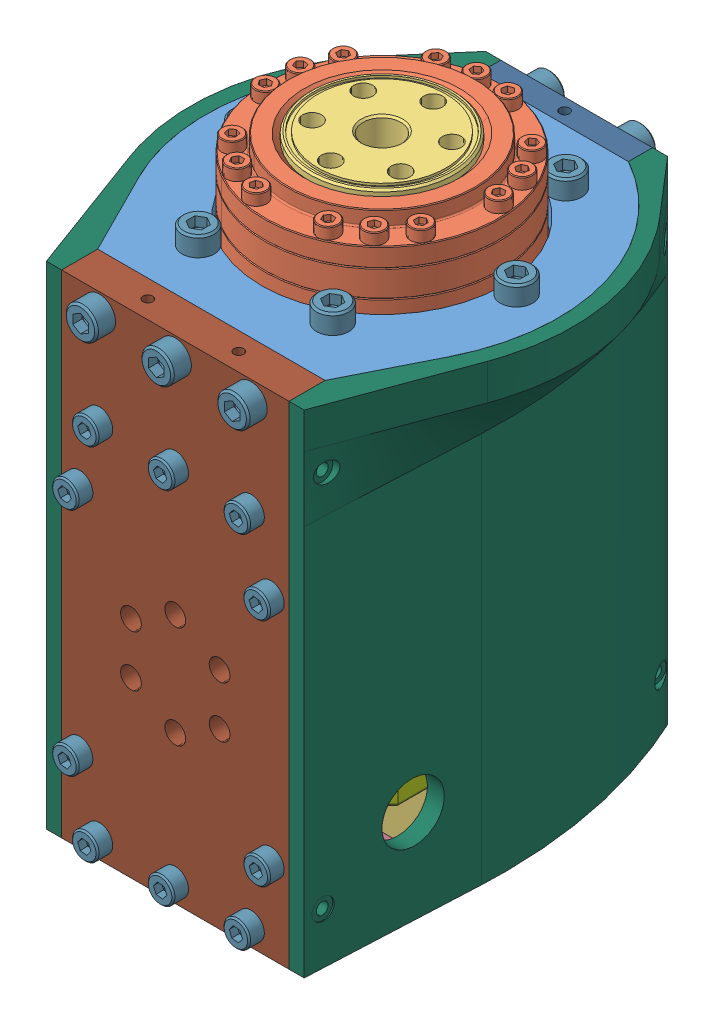
SolidWorks assembly DEC_asm, configuration Default. Lengths in mm.
Overall size (107.92 151.34 115.88).
57 component instances, 15 part files, 101 mates.
Components (placement in the parent):
- DEC_gearbox_mount-1: DEC_gearbox_mount [Default] at (31.2065 45.5966 71.2738) size (92.96 9.53 90)
- CSF-17-XXX-2UH.stp-1: CSF-17-XXX-2UH.stp [Default] at (31.2065 69.8341 71.2738) x (0 -1 0) z (0.5 0 -0.866025) size (45 79 79)
  - CSF-17-2UH HOUSING.stp-1: CSF-17-2UH HOUSING.stp [Default] at origin size (38.5 79 79)
  - CSF-17-2UH OUTPUT.stp-1: CSF-17-2UH OUTPUT.stp [Default] at (0 -0.0003 0) x (1 0.000008 0) z (0 0 1) size (39 44 44)
  - CSF-17-2A-R OLDHAM COUPLING.stp-1: CSF-17-2A-R OLDHAM COUPLING.stp [Default] at (45 0 0) x (1 0 0) z (0 0 -1) size (19.5 37 37)
  - 1715063_1715063.stp-1: 1715063_1715063.stp [Default] at (42 0 9) x (0 0 -1) z (-0.999997 -0.002366 0) size (4 3 3)
  - 1715063_1715063.stp-2: 1715063_1715063.stp [Default] at (42 -9 0) x (0 1 0) z (0.378269 0 0.925696) size (4 3 3)
  - 17 WG BEARING.stp-1: 17 WG BEARING.stp [Default] at (32.285 0 0) size (6.67 42 42)
- Nema17_27_1-1: Nema17_27_1 [Default] at (-8.1003 -74.3741 116.9592) x (1 0 0) z (0 1 0) size (42.4 43.16 103.01)
  - 6627T91_Stepper Motor-1: 6627T91_Stepper Motor [6627T91] at (39.3069 45.6854 45.8837) size (42.4 43.16 74.04)
  - Planatary_Gearbox_27_1-1: Planatary_Gearbox_27_1 [Default] at (39.3069 45.6854 56.8707) size (42.1 42.1 55)
- DEC_planetary_mount-1: DEC_planetary_mount [Default] at (31.2065 20.5966 71.2738) x (1 0 0) z (0 1 0) size (60 90 6.2)
- DEC_top_plate-1: DEC_top_plate [Default] at (31.2065 -29.6409 23.0988) x (-1 0 0) z (0 -1 0) size (40 6.35 129.76)
- DEC_bottom_plate-1: DEC_bottom_plate [Default] at (31.2065 -29.6409 121.0388) x (-1 0 0) z (0 -1 0) size (60 9.53 129.76)
- DEC_middle_support_v2-1: DEC_middle_support_v2 [Default] at (31.2065 -74.4034 71.2738) x (-1 0 0) z (0 -1 0) size (60 90 6.2)
- support_triangle-1: support_triangle [Default] at (51.6815 -71.3034 116.2738) x (0 0 -1) z (1 0 0) size (18 18 9.53)
- support_triangle-2: support_triangle [Default] at (41.6815 -71.3034 26.2738) x (0 1 0) z (1 0 0) size (18 18 9.53)
- support_triangle-3: support_triangle [Default] at (1.2065 -71.3034 116.2738) x (0 0 -1) z (1 0 0) size (18 18 9.53)
- support_triangle-4: support_triangle [Default] at (11.2065 -71.3034 26.2738) x (0 1 0) z (1 0 0) size (18 18 9.53)
- support_triangle-5: support_triangle [Default] at (41.6815 17.4966 26.2738) x (0 0 1) z (1 0 0) size (18 18 9.53)
- support_triangle-6: support_triangle [Default] at (1.2065 17.4966 116.2738) x (0 -1 0) z (1 0 0) size (18 18 9.53)
- support_triangle-7: support_triangle [Default] at (51.6815 17.4966 116.2738) x (0 -1 0) z (1 0 0) size (18 18 9.53)
- support_triangle-8: support_triangle [Default] at (11.2065 17.4966 26.2738) x (0 0 1) z (1 0 0) size (18 18 9.53)
- socket head cap screw_am-4: socket head cap screw_am [B18.3.1M - 4 x 0.7 x 12 Hex SHCS -- 12NHX] at (43.2065 -74.4034 15.9238) x (0 0 1) z (-1 0 0) size (16 7 7)
- socket head cap screw_am-5: socket head cap screw_am [B18.3.1M - 4 x 0.7 x 12 Hex SHCS -- 12NHX] at (19.2065 20.5966 15.9238) x (0 0 1) z (-0.77104 0.636787 0) size (16 7 7)
- socket head cap screw_am-6: socket head cap screw_am [B18.3.1M - 4 x 0.7 x 12 Hex SHCS -- 12NHX] at (46.444 -57.3034 15.9238) x (0 0 1) z (-1 0 0) size (16 7 7)
- socket head cap screw_am-7: socket head cap screw_am [B18.3.1M - 4 x 0.7 x 12 Hex SHCS -- 12NHX] at (19.2065 -74.4034 15.9238) x (0 0 1) z (-1 0 0) size (16 7 7)
- socket head cap screw_am-8: socket head cap screw_am [B18.3.1M - 4 x 0.7 x 12 Hex SHCS -- 12NHX] at (15.969 3.4966 15.9238) x (0 0 1) z (-1 0 0) size (16 7 7)
- socket head cap screw_am-9: socket head cap screw_am [B18.3.1M - 4 x 0.7 x 12 Hex SHCS -- 12NHX] at (15.969 -57.3034 15.9238) x (0 0 1) z (-1 0 0) size (16 7 7)
- socket head cap screw_am-10: socket head cap screw_am [B18.3.1M - 4 x 0.7 x 12 Hex SHCS -- 12NHX] at (43.2065 20.5966 15.9238) x (0 0 1) z (-1 0 0) size (16 7 7)
- socket head cap screw_am-11: socket head cap screw_am [B18.3.1M - 4 x 0.7 x 12 Hex SHCS -- 12NHX] at (46.444 3.4966 15.9238) x (0 0 1) z (-1 0 0) size (16 7 7)
- socket head cap screw_am-12: socket head cap screw_am [B18.3.1M - 5 x 0.8 x 12 Hex SHCS -- 12NHX] at (43.2065 45.5966 14.9238) x (0 0 1) z (-1 0 0) size (17 8.5 8.5)
- socket head cap screw_am-13: socket head cap screw_am [B18.3.1M - 5 x 0.8 x 12 Hex SHCS -- 12NHX] at (19.2065 45.5966 14.9238) x (0 0 1) z (-1 0 0) size (17 8.5 8.5)
- socket head cap screw_am-14: socket head cap screw_am [B18.3.1M - 5 x 0.8 x 12 Hex SHCS -- 12NHX] at (51.2065 45.5966 130.8038) x (0 0 -1) z (1 0 0) size (17 8.5 8.5)
- socket head cap screw_am-15: socket head cap screw_am [B18.3.1M - 5 x 0.8 x 12 Hex SHCS -- 12NHX] at (11.2065 45.5966 130.8038) x (0 0 -1) z (1 0 0) size (17 8.5 8.5)
- socket head cap screw_am-16: socket head cap screw_am [B18.3.1M - 5 x 0.8 x 12 Hex SHCS -- 12NHX] at (31.2065 45.5966 130.8038) x (0 0 -1) z (1 0 0) size (17 8.5 8.5)
- socket head cap screw_am-17: socket head cap screw_am [B18.3.1M - 4 x 0.7 x 12 Hex SHCS -- 12NHX] at (31.2065 20.5966 129.8038) x (0 0 -1) z (0.923728 0.383049 0) size (16 7 7)
- socket head cap screw_am-18: socket head cap screw_am [B18.3.1M - 4 x 0.7 x 12 Hex SHCS -- 12NHX] at (51.2065 20.5966 129.8038) x (0 0 -1) z (0.923728 0.383049 0) size (16 7 7)
- socket head cap screw_am-19: socket head cap screw_am [B18.3.1M - 4 x 0.7 x 12 Hex SHCS -- 12NHX] at (5.969 3.4966 129.8038) x (0 0 -1) z (0.923728 0.383049 0) size (16 7 7)
- socket head cap screw_am-20: socket head cap screw_am [B18.3.1M - 4 x 0.7 x 12 Hex SHCS -- 12NHX] at (56.444 3.4966 129.8038) x (0 0 -1) z (0.923728 0.383049 0) size (16 7 7)
- socket head cap screw_am-21: socket head cap screw_am [B18.3.1M - 4 x 0.7 x 12 Hex SHCS -- 12NHX] at (5.969 -57.3034 129.8038) x (0 0 -1) z (0.923728 0.383049 0) size (16 7 7)
- socket head cap screw_am-22: socket head cap screw_am [B18.3.1M - 4 x 0.7 x 12 Hex SHCS -- 12NHX] at (56.444 -57.3034 129.8038) x (0 0 -1) z (0.923728 0.383049 0) size (16 7 7)
- socket head cap screw_am-23: socket head cap screw_am [B18.3.1M - 4 x 0.7 x 12 Hex SHCS -- 12NHX] at (11.2065 -74.4034 129.8038) x (0 0 -1) z (0.923728 0.383049 0) size (16 7 7)
- socket head cap screw_am-24: socket head cap screw_am [B18.3.1M - 4 x 0.7 x 12 Hex SHCS -- 12NHX] at (51.2065 -74.4034 129.8038) x (0 0 -1) z (0.923728 0.383049 0) size (16 7 7)
- socket head cap screw_am-25: socket head cap screw_am [B18.3.1M - 4 x 0.7 x 12 Hex SHCS -- 12NHX] at (11.2065 20.5966 129.8038) x (0 0 -1) z (0.923728 0.383049 0) size (16 7 7)
- socket head cap screw_am-26: socket head cap screw_am [B18.3.1M - 4 x 0.7 x 12 Hex SHCS -- 12NHX] at (31.2065 -74.4034 129.8038) x (0 0 -1) z (0.923728 0.383049 0) size (16 7 7)
- socket head cap screw_am-27: socket head cap screw_am [B18.3.1M - 4 x 0.7 x 12 Hex SHCS -- 12NHX] at (46.444 -81.5034 40.2738) x (0 1 0) z (-0.56381 0 -0.825904) size (16 7 7)
- socket head cap screw_am-28: socket head cap screw_am [B18.3.1M - 4 x 0.7 x 12 Hex SHCS -- 12NHX] at (15.969 -81.5034 40.2738) x (0 1 0) z (-0.56381 0 -0.825904) size (16 7 7)
- socket head cap screw_am-29: socket head cap screw_am [B18.3.1M - 4 x 0.7 x 12 Hex SHCS -- 12NHX] at (5.969 -81.5034 102.2738) x (0 1 0) z (-0.56381 0 -0.825904) size (16 7 7)
- socket head cap screw_am-30: socket head cap screw_am [B18.3.1M - 4 x 0.7 x 12 Hex SHCS -- 12NHX] at (56.444 -81.5034 102.2738) x (0 1 0) z (-0.56381 0 -0.825904) size (16 7 7)
- socket head cap screw_am-31: socket head cap screw_am [B18.3.1M - 5 x 0.8 x 12 Hex SHCS -- 12NHX] at (48.9565 55.3591 102.0177) x (0 -1 0) z (1 0 0) size (17 8.5 8.5)
- socket head cap screw_am-32: socket head cap screw_am [B18.3.1M - 5 x 0.8 x 12 Hex SHCS -- 12NHX] at (13.4565 55.3591 102.0177) x (0 -1 0) z (1 0 0) size (17 8.5 8.5)
- socket head cap screw_am-33: socket head cap screw_am [B18.3.1M - 5 x 0.8 x 12 Hex SHCS -- 12NHX] at (48.9565 55.3591 40.5299) x (0 -1 0) z (1 0 0) size (17 8.5 8.5)
- socket head cap screw_am-34: socket head cap screw_am [B18.3.1M - 5 x 0.8 x 12 Hex SHCS -- 12NHX] at (-4.2935 55.3591 71.2738) x (0 -1 0) z (1 0 0) size (17 8.5 8.5)
- socket head cap screw_am-35: socket head cap screw_am [B18.3.1M - 5 x 0.8 x 12 Hex SHCS -- 12NHX] at (13.4565 55.3591 40.5299) x (0 -1 0) z (1 0 0) size (17 8.5 8.5)
- socket head cap screw_am-36: socket head cap screw_am [B18.3.1M - 5 x 0.8 x 12 Hex SHCS -- 12NHX] at (66.7065 55.3591 71.2738) x (0 -1 0) z (1 0 0) size (17 8.5 8.5)
- Part1^DEC_asm-1: Part1^DEC_asm [Default] at origin size (101.02 129.76 105.9) (virtual)
Mates (geometry in assembly coordinates):
- Coincident3: coincident anti-aligned: plane of RA_gearbox_mount-1 through (11.2065 50.3591 26.2738) normal (0 0 -1); plane of DEC_top_plate-1 through (31.2065 -29.6409 26.2738) normal (0 0 1)
- Concentric8: concentric aligned: cylinder of RA_gearbox_mount-1 through (31.2065 45.5966 108.2738) axis (0 0 1) radius 2.15; cylinder of DEC_bottom_plate-1 through (31.2065 45.5966 114.6888) axis (0 0 1) radius 2.75
- Concentric9: concentric aligned: cylinder of RA_planetary_mount-1 through (31.2065 20.5966 108.2738) axis (0 0 1) radius 1.7; cylinder of DEC_bottom_plate-1 through (31.2065 20.5966 114.6888) axis (0 0 1) radius 2.2
- Coincident4: coincident anti-aligned: plane of RA_planetary_mount-1 through (1.2065 23.6966 116.2738) normal (0 0 1); plane of DEC_bottom_plate-1 through (31.2065 -29.6409 116.2738) normal (0 0 -1)
- Concentric10: concentric aligned: cylinder of DEC_bottom_plate-1 through (11.2065 -74.4034 114.6888) axis (0 0 1) radius 2.2; cylinder of DEC_middle_support_v2-1 through (11.2065 -74.4034 108.2738) axis (0 0 1) radius 1.7
- Concentric11: concentric aligned: cylinder of DEC_bottom_plate-1 through (51.2065 -74.4034 114.6888) axis (0 0 1) radius 2.2; cylinder of DEC_middle_support_v2-1 through (51.2065 -74.4034 108.2738) axis (0 0 1) radius 1.7
- Coincident5: coincident anti-aligned: plane of DEC_bottom_plate-1 through (31.2065 -29.6409 116.2738) normal (0 0 -1); plane of DEC_middle_support_v2-1 through (61.2065 -77.5034 116.2738) normal (0 0 1)
- Concentric14: concentric anti-aligned: cylinder of RA_gearbox_mount-1 through (43.2065 45.5966 34.2738) axis (0 0 -1) radius 2.15; cylinder of DEC_top_plate-1 through (43.2065 45.5966 16.7488) axis (0 0 1) radius 2.75
- Concentric15: concentric anti-aligned: cylinder of RA_planetary_mount-1 through (19.2065 20.5966 34.2738) axis (0 0 -1) radius 1.7; cylinder of DEC_top_plate-1 through (19.2065 20.5966 16.7488) axis (0 0 1) radius 2.2
- Coincident6: coincident anti-aligned: plane of RA_gearbox_mount-1 through (26.2065 40.8341 71.2738) normal (0 -1 0); plane of CSF-17-XXX-2UH.stp-1/CSF-17-2UH HOUSING.stp-1 through (3.5803 40.8341 55.3238) normal (0 1 0)
- Concentric16: concentric anti-aligned: cylinder of RA_gearbox_mount-1 through (13.4565 34.6116 40.5299) axis (0 1 0) radius 2.2; cylinder of CSF-17-XXX-2UH.stp-1/CSF-17-2UH HOUSING.stp-1 through (13.4565 32.8341 40.5299) axis (0 -1 0) radius 1.65
- Concentric18: concentric anti-aligned: cylinder of RA_gearbox_mount-1 through (-4.2935 34.6116 71.2738) axis (0 1 0) radius 2.2; cylinder of CSF-17-XXX-2UH.stp-1/CSF-17-2UH HOUSING.stp-1 through (-4.2935 32.8341 71.2738) axis (0 -1 0) radius 1.65
- Concentric19: concentric anti-aligned: cylinder of RA_gearbox_mount-1 through (19.2065 45.5966 34.2738) axis (0 0 -1) radius 2.15; cylinder of DEC_top_plate-1 through (19.2065 45.5966 16.7488) axis (0 0 1) radius 2.75
- Coincident7: coincident anti-aligned: plane of RA_planetary_mount-1 through (11.2065 23.6966 26.2738) normal (0 0 -1); plane of DEC_top_plate-1 through (31.2065 -29.6409 26.2738) normal (0 0 1)
- Concentric20: concentric anti-aligned: cylinder of DEC_top_plate-1 through (19.2065 -74.4034 16.7488) axis (0 0 1) radius 2.2; cylinder of DEC_middle_support_v2-1 through (19.2065 -74.4034 34.2738) axis (0 0 -1) radius 1.7
- Concentric21: concentric anti-aligned: cylinder of DEC_top_plate-1 through (43.2065 -74.4034 16.7488) axis (0 0 1) radius 2.2; cylinder of DEC_middle_support_v2-1 through (43.2065 -74.4034 34.2738) axis (0 0 -1) radius 1.7
- Concentric22: concentric aligned: cylinder of Nema17_27_1-1/Planatary_Gearbox_27_1-1 through (21.307 7.4966 61.3743) axis (0 1 0) radius 1.5; cylinder of RA_planetary_mount-1 through (21.307 13.8196 61.3743) axis (0 1 0) radius 1.3
- Concentric283: concentric aligned: circle of Nema17_27_1-1/Planatary_Gearbox_27_1-1; cylinder of DEC_planetary_mount-1 through (21.307 13.8196 81.1733) axis (0 1 0) radius 1.3
- Coincident9: coincident anti-aligned: plane of Nema17_27_1-1/Planatary_Gearbox_27_1-1 through (31.2065 17.4966 71.2738) normal (0 1 0); plane of RA_planetary_mount-1 through (31.2065 17.4966 71.2738) normal (0 -1 0)
- Concentric23: concentric anti-aligned: cylinder of DEC_bottom_plate-1 through (56.444 -57.3034 132.0264) axis (0 0 -1) radius 2.2; cylinder of support_triangle-1 through (56.444 -57.3034 102.617) axis (0 0 1) radius 2
- Concentric24: concentric aligned: cylinder of DEC_middle_support_v2-1 through (56.444 -65.0809 102.2738) axis (0 -1 0) radius 2.2; cylinder of support_triangle-1 through (56.444 -57.6465 102.2738) axis (0 -1 0) radius 2
- Concentric25: concentric anti-aligned: circle of RA_middle_support-1; cylinder of support_triangle-2 through (46.444 -57.6465 40.2738) axis (0 -1 0) radius 2
- Concentric26: concentric aligned: cylinder of DEC_top_plate-1 through (46.444 -57.3034 32.4964) axis (0 0 -1) radius 2.2; cylinder of support_triangle-2 through (46.444 -57.3034 39.9307) axis (0 0 -1) radius 2
- Concentric27: concentric anti-aligned: cylinder of DEC_bottom_plate-1 through (5.969 -57.3034 132.0264) axis (0 0 -1) radius 2.2; cylinder of support_triangle-3 through (5.969 -57.3034 102.617) axis (0 0 1) radius 2
- Concentric28: concentric aligned: cylinder of DEC_middle_support_v2-1 through (5.969 -65.0809 102.2738) axis (0 -1 0) radius 2.2; cylinder of support_triangle-3 through (5.969 -57.6465 102.2738) axis (0 -1 0) radius 2
- Concentric29: concentric aligned: cylinder of DEC_top_plate-1 through (15.969 -57.3034 32.4964) axis (0 0 -1) radius 2.2; cylinder of support_triangle-4 through (15.969 -57.3034 39.9307) axis (0 0 -1) radius 2
- Concentric30: concentric aligned: cylinder of DEC_middle_support_v2-1 through (15.969 -65.0809 40.2738) axis (0 -1 0) radius 2.2; cylinder of support_triangle-4 through (15.969 -57.6465 40.2738) axis (0 -1 0) radius 2
- Concentric31: concentric anti-aligned: cylinder of RA_planetary_mount-1 through (5.969 11.2741 102.2738) axis (0 1 0) radius 2.2; circle of support_triangle-6
- Concentric32: concentric anti-aligned: cylinder of DEC_bottom_plate-1 through (5.969 3.4966 132.0264) axis (0 0 -1) radius 2.2; circle of support_triangle-6
- Concentric33: concentric anti-aligned: cylinder of DEC_bottom_plate-1 through (56.444 3.4966 132.0264) axis (0 0 -1) radius 2.2; circle of support_triangle-7
- Concentric34: concentric aligned: cylinder of RA_planetary_mount-1 through (56.444 11.2741 102.2738) axis (0 1 0) radius 2.2; cylinder of support_triangle-7 through (56.444 3.8397 102.2738) axis (0 1 0) radius 2
- Concentric36: concentric aligned: cylinder of RA_planetary_mount-1 through (46.444 11.2741 40.2738) axis (0 1 0) radius 2.2; cylinder of support_triangle-5 through (46.444 3.8397 40.2738) axis (0 1 0) radius 2
- Concentric37: concentric aligned: cylinder of DEC_top_plate-1 through (46.444 3.4966 32.4964) axis (0 0 -1) radius 2.2; circle of support_triangle-5
- Concentric38: concentric aligned: cylinder of DEC_top_plate-1 through (15.969 3.4966 32.4964) axis (0 0 -1) radius 2.2; cylinder of support_triangle-8 through (15.969 3.4966 39.9307) axis (0 0 -1) radius 2
- Concentric39: concentric anti-aligned: cylinder of RA_planetary_mount-1 through (15.969 11.2741 40.2738) axis (0 1 0) radius 2.2; circle of support_triangle-8
- Concentric250: concentric anti-aligned: cylinder of DEC_top_plate-1 through (19.2065 20.5966 16.7488) axis (0 0 1) radius 2.2; cylinder of socket head cap screw_am-5 through (19.2065 20.5966 -15.8262) axis (0 0 -1) radius 2
- Coincident219: coincident aligned: plane of DEC_top_plate-1 through (31.2065 -29.6409 19.9238) normal (0 0 -1); circle of socket head cap screw_am-5
- Coincident220: coincident aligned: plane of socket head cap screw_am-4 through (43.2065 -72.7934 31.9238) normal (0 0 1); plane of socket head cap screw_am-7 through (19.2065 -72.7934 31.9238) normal (0 0 1)
- Coincident221: coincident aligned: plane of socket head cap screw_am-6 through (46.444 -55.6934 31.9238) normal (0 0 1); plane of socket head cap screw_am-7 through (19.2065 -72.7934 31.9238) normal (0 0 1)
- Coincident222: coincident aligned: plane of socket head cap screw_am-6 through (46.444 -55.6934 31.9238) normal (0 0 1); plane of socket head cap screw_am-9 through (15.969 -55.6934 31.9238) normal (0 0 1)
- Coincident223: coincident aligned: plane of socket head cap screw_am-9 through (15.969 -55.6934 31.9238) normal (0 0 1); plane of socket head cap screw_am-11 through (46.444 5.1066 31.9238) normal (0 0 1)
- Coincident224: coincident aligned: plane of socket head cap screw_am-8 through (15.969 5.1066 31.9238) normal (0 0 1); plane of socket head cap screw_am-11 through (46.444 5.1066 31.9238) normal (0 0 1)
- Coincident225: coincident aligned: plane of socket head cap screw_am-8 through (15.969 5.1066 31.9238) normal (0 0 1); plane of socket head cap screw_am-10 through (43.2065 22.2066 31.9238) normal (0 0 1)
- Coincident226: coincident anti-aligned: plane of DEC_top_plate-1 through (31.2065 -29.6409 19.9238) normal (0 0 -1); plane of socket head cap screw_am-10 through (43.2065 24.0966 19.9238) normal (0 0 1)
- Concentric251: concentric anti-aligned: circle of DEC_top_plate-1; cylinder of socket head cap screw_am-10 through (43.2065 20.5966 -15.8262) axis (0 0 -1) radius 3.5
- Concentric252: concentric aligned: circle of DEC_top_plate-1; cylinder of socket head cap screw_am-8 through (15.969 3.4966 -15.8262) axis (0 0 -1) radius 2
- Concentric253: concentric aligned: cylinder of DEC_top_plate-1 through (46.444 3.4966 32.4964) axis (0 0 -1) radius 2.2; cylinder of socket head cap screw_am-11 through (46.444 3.4966 -15.8262) axis (0 0 -1) radius 2
- Concentric254: concentric aligned: circle of DEC_top_plate-1; cylinder of socket head cap screw_am-9 through (15.969 -57.3034 -15.8262) axis (0 0 -1) radius 2
- Concentric255: concentric aligned: cylinder of DEC_top_plate-1 through (46.444 -57.3034 32.4964) axis (0 0 -1) radius 2.2; cylinder of socket head cap screw_am-6 through (46.444 -57.3034 -15.8262) axis (0 0 -1) radius 2
- Concentric256: concentric anti-aligned: circle of DEC_top_plate-1; cylinder of socket head cap screw_am-7 through (19.2065 -74.4034 -15.8262) axis (0 0 -1) radius 2
- Concentric257: concentric anti-aligned: circle of DEC_top_plate-1; cylinder of socket head cap screw_am-4 through (43.2065 -74.4034 -15.8262) axis (0 0 -1) radius 2
- Coincident227: coincident aligned: plane of socket head cap screw_am-12 through (43.2065 47.6516 31.9238) normal (0 0 1); plane of socket head cap screw_am-13 through (19.2065 47.6516 31.9238) normal (0 0 1)
- Coincident228: coincident anti-aligned: plane of DEC_top_plate-1 through (31.2065 -29.6409 19.9238) normal (0 0 -1); plane of socket head cap screw_am-13 through (19.2065 49.8466 19.9238) normal (0 0 1)
- Concentric258: concentric anti-aligned: cylinder of DEC_top_plate-1 through (19.2065 45.5966 16.7488) axis (0 0 1) radius 2.75; cylinder of socket head cap screw_am-13 through (19.2065 45.5966 -16.8262) axis (0 0 -1) radius 4.25
- Concentric259: concentric anti-aligned: cylinder of DEC_top_plate-1 through (43.2065 45.5966 16.7488) axis (0 0 1) radius 2.75; cylinder of socket head cap screw_am-12 through (43.2065 45.5966 -16.8262) axis (0 0 -1) radius 2.5
- Coincident229: coincident aligned: plane of socket head cap screw_am-15 through (11.2065 47.6516 113.8038) normal (0 0 -1); plane of socket head cap screw_am-16 through (31.2065 47.6516 113.8038) normal (0 0 -1)
- Coincident230: coincident aligned: plane of socket head cap screw_am-14 through (51.2065 47.6516 113.8038) normal (0 0 -1); plane of socket head cap screw_am-15 through (11.2065 47.6516 113.8038) normal (0 0 -1)
- Coincident231: coincident anti-aligned: plane of DEC_bottom_plate-1 through (31.2065 -29.6409 125.8038) normal (0 0 1); plane of socket head cap screw_am-14 through (51.2065 49.8466 125.8038) normal (0 0 -1)
- Concentric260: concentric aligned: cylinder of DEC_bottom_plate-1 through (51.2065 45.5966 114.6888) axis (0 0 1) radius 2.75; cylinder of socket head cap screw_am-14 through (51.2065 45.5966 162.5538) axis (0 0 1) radius 2.5
- Concentric261: concentric aligned: cylinder of DEC_bottom_plate-1 through (31.2065 45.5966 114.6888) axis (0 0 1) radius 2.75; cylinder of socket head cap screw_am-16 through (31.2065 45.5966 162.5538) axis (0 0 1) radius 2.5
- Concentric262: concentric aligned: cylinder of DEC_bottom_plate-1 through (11.2065 45.5966 114.6888) axis (0 0 1) radius 2.75; cylinder of socket head cap screw_am-15 through (11.2065 45.5966 162.5538) axis (0 0 1) radius 2.5
- Coincident232: coincident aligned: plane of socket head cap screw_am-17 through (30.5898 22.0838 113.8038) normal (0 0 -1); plane of socket head cap screw_am-18 through (50.5898 22.0838 113.8038) normal (0 0 -1)
- Coincident233: coincident aligned: plane of socket head cap screw_am-18 through (50.5898 22.0838 113.8038) normal (0 0 -1); plane of socket head cap screw_am-19 through (5.3523 4.9838 113.8038) normal (0 0 -1)
- Coincident234: coincident aligned: plane of socket head cap screw_am-18 through (50.5898 22.0838 113.8038) normal (0 0 -1); plane of socket head cap screw_am-20 through (55.8273 4.9838 113.8038) normal (0 0 -1)
- Coincident235: coincident aligned: plane of socket head cap screw_am-20 through (55.8273 4.9838 113.8038) normal (0 0 -1); plane of socket head cap screw_am-21 through (5.3523 -55.8162 113.8038) normal (0 0 -1)
- Coincident236: coincident aligned: plane of socket head cap screw_am-21 through (5.3523 -55.8162 113.8038) normal (0 0 -1); plane of socket head cap screw_am-22 through (55.8273 -55.8162 113.8038) normal (0 0 -1)
- Coincident237: coincident aligned: plane of socket head cap screw_am-22 through (55.8273 -55.8162 113.8038) normal (0 0 -1); plane of socket head cap screw_am-23 through (10.5898 -72.9162 113.8038) normal (0 0 -1)
- Coincident238: coincident aligned: plane of socket head cap screw_am-23 through (10.5898 -72.9162 113.8038) normal (0 0 -1); plane of socket head cap screw_am-26 through (30.5898 -72.9162 113.8038) normal (0 0 -1)
- Coincident239: coincident aligned: plane of socket head cap screw_am-24 through (50.5898 -72.9162 113.8038) normal (0 0 -1); plane of socket head cap screw_am-26 through (30.5898 -72.9162 113.8038) normal (0 0 -1)
- Coincident240: coincident aligned: plane of socket head cap screw_am-24 through (50.5898 -72.9162 113.8038) normal (0 0 -1); plane of socket head cap screw_am-25 through (10.5898 22.0838 113.8038) normal (0 0 -1)
- Coincident241: coincident anti-aligned: plane of DEC_bottom_plate-1 through (31.2065 -29.6409 125.8038) normal (0 0 1); plane of socket head cap screw_am-25 through (9.8659 23.8296 125.8038) normal (0 0 -1)
- Concentric263: concentric aligned: cylinder of DEC_bottom_plate-1 through (11.2065 20.5966 114.6888) axis (0 0 1) radius 2.2; cylinder of socket head cap screw_am-25 through (11.2065 20.5966 161.5538) axis (0 0 1) radius 3.5
- Concentric264: concentric aligned: cylinder of DEC_bottom_plate-1 through (31.2065 20.5966 114.6888) axis (0 0 1) radius 2.2; cylinder of socket head cap screw_am-17 through (31.2065 20.5966 161.5538) axis (0 0 1) radius 2
- Concentric265: concentric aligned: cylinder of DEC_bottom_plate-1 through (51.2065 20.5966 114.6888) axis (0 0 1) radius 2.2; cylinder of socket head cap screw_am-18 through (51.2065 20.5966 161.5538) axis (0 0 1) radius 2
- Concentric266: concentric anti-aligned: cylinder of DEC_bottom_plate-1 through (5.969 3.4966 132.0264) axis (0 0 -1) radius 2.2; cylinder of socket head cap screw_am-19 through (5.969 3.4966 161.5538) axis (0 0 1) radius 2
- Concentric267: concentric anti-aligned: cylinder of DEC_bottom_plate-1 through (56.444 3.4966 132.0264) axis (0 0 -1) radius 2.2; cylinder of socket head cap screw_am-20 through (56.444 3.4966 161.5538) axis (0 0 1) radius 2
- Concentric268: concentric anti-aligned: cylinder of DEC_bottom_plate-1 through (5.969 -57.3034 132.0264) axis (0 0 -1) radius 2.2; cylinder of socket head cap screw_am-21 through (5.969 -57.3034 161.5538) axis (0 0 1) radius 2
- Concentric269: concentric anti-aligned: cylinder of DEC_bottom_plate-1 through (56.444 -57.3034 132.0264) axis (0 0 -1) radius 2.2; cylinder of socket head cap screw_am-22 through (56.444 -57.3034 161.5538) axis (0 0 1) radius 2
- Concentric270: concentric aligned: cylinder of DEC_bottom_plate-1 through (11.2065 -74.4034 114.6888) axis (0 0 1) radius 2.2; cylinder of socket head cap screw_am-23 through (11.2065 -74.4034 161.5538) axis (0 0 1) radius 2
- Concentric271: concentric aligned: cylinder of DEC_bottom_plate-1 through (31.2065 -74.4034 114.6888) axis (0 0 1) radius 2.2; cylinder of socket head cap screw_am-26 through (31.2065 -74.4034 161.5538) axis (0 0 1) radius 2
- Concentric272: concentric aligned: cylinder of DEC_bottom_plate-1 through (51.2065 -74.4034 114.6888) axis (0 0 1) radius 2.2; cylinder of socket head cap screw_am-24 through (51.2065 -74.4034 161.5538) axis (0 0 1) radius 2
- Concentric273: concentric aligned: cylinder of DEC_middle_support_v2-1 through (46.444 -65.0809 40.2738) axis (0 -1 0) radius 2.2; cylinder of socket head cap screw_am-27 through (46.444 -113.2534 40.2738) axis (0 -1 0) radius 2
- Coincident242: coincident anti-aligned: plane of DEC_middle_support_v2-1 through (31.2065 -77.5034 71.2738) normal (0 -1 0); plane of socket head cap screw_am-27 through (49.3347 -77.5034 38.3005) normal (0 1 0)
- Coincident243: coincident aligned: plane of socket head cap screw_am-28 through (17.2987 -65.5034 39.3661) normal (0 1 0); plane of socket head cap screw_am-29 through (7.2987 -65.5034 101.3661) normal (0 1 0)
- Coincident244: coincident aligned: plane of socket head cap screw_am-29 through (7.2987 -65.5034 101.3661) normal (0 1 0); plane of socket head cap screw_am-30 through (57.7737 -65.5034 101.3661) normal (0 1 0)
- Coincident245: coincident aligned: plane of socket head cap screw_am-27 through (46.444 -81.5034 40.2738) normal (0 -1 0); plane of socket head cap screw_am-28 through (15.969 -81.5034 40.2738) normal (0 -1 0)
- Concentric274: concentric aligned: cylinder of DEC_middle_support_v2-1 through (15.969 -65.0809 40.2738) axis (0 -1 0) radius 2.2; cylinder of socket head cap screw_am-28 through (15.969 -113.2534 40.2738) axis (0 -1 0) radius 3.5
- Concentric275: concentric aligned: cylinder of DEC_middle_support_v2-1 through (5.969 -65.0809 102.2738) axis (0 -1 0) radius 2.2; cylinder of socket head cap screw_am-29 through (5.969 -113.2534 102.2738) axis (0 -1 0) radius 2
- Concentric276: concentric aligned: cylinder of DEC_middle_support_v2-1 through (56.444 -65.0809 102.2738) axis (0 -1 0) radius 2.2; cylinder of socket head cap screw_am-30 through (56.444 -113.2534 102.2738) axis (0 -1 0) radius 2
- Coincident246: coincident aligned: plane of socket head cap screw_am-32 through (13.4565 38.3591 99.9627) normal (0 -1 0); plane of socket head cap screw_am-33 through (48.9565 38.3591 38.4749) normal (0 -1 0)
- Coincident247: coincident aligned: plane of socket head cap screw_am-33 through (48.9565 38.3591 38.4749) normal (0 -1 0); plane of socket head cap screw_am-34 through (-4.2935 38.3591 69.2188) normal (0 -1 0)
- Coincident248: coincident aligned: plane of socket head cap screw_am-31 through (48.9565 38.3591 99.9627) normal (0 -1 0); plane of socket head cap screw_am-32 through (13.4565 38.3591 99.9627) normal (0 -1 0)
- Coincident249: coincident aligned: plane of socket head cap screw_am-31 through (48.9565 38.3591 99.9627) normal (0 -1 0); plane of socket head cap screw_am-36 through (66.7065 38.3591 69.2188) normal (0 -1 0)
- Coincident250: coincident aligned: plane of socket head cap screw_am-35 through (13.4565 38.3591 38.4749) normal (0 -1 0); plane of socket head cap screw_am-36 through (66.7065 38.3591 69.2188) normal (0 -1 0)
- Coincident251: coincident anti-aligned: plane of DEC_gearbox_mount-1 through (26.2065 50.3591 71.2738) normal (0 1 0); plane of socket head cap screw_am-35 through (13.4565 50.3591 36.2799) normal (0 -1 0)
- Concentric277: concentric aligned: cylinder of DEC_gearbox_mount-1 through (13.4565 34.6116 40.5299) axis (0 1 0) radius 2.2; cylinder of socket head cap screw_am-35 through (13.4565 87.1091 40.5299) axis (0 1 0) radius 2.5
- Concentric278: concentric aligned: cylinder of DEC_gearbox_mount-1 through (-4.2935 34.6116 71.2738) axis (0 1 0) radius 2.2; cylinder of socket head cap screw_am-34 through (-4.2935 87.1091 71.2738) axis (0 1 0) radius 2.5
- Concentric279: concentric aligned: cylinder of DEC_gearbox_mount-1 through (48.9565 34.6116 40.5299) axis (0 1 0) radius 2.2; cylinder of socket head cap screw_am-33 through (48.9565 87.1091 40.5299) axis (0 1 0) radius 2.5
- Concentric280: concentric aligned: cylinder of DEC_gearbox_mount-1 through (66.7065 34.6116 71.2738) axis (0 1 0) radius 2.2; cylinder of socket head cap screw_am-36 through (66.7065 87.1091 71.2738) axis (0 1 0) radius 2.5
- Concentric281: concentric aligned: cylinder of DEC_gearbox_mount-1 through (48.9565 34.6116 102.0177) axis (0 1 0) radius 2.2; cylinder of socket head cap screw_am-31 through (48.9565 87.1091 102.0177) axis (0 1 0) radius 2.5
- Concentric282: concentric aligned: cylinder of DEC_gearbox_mount-1 through (13.4565 34.6116 102.0177) axis (0 1 0) radius 2.2; cylinder of socket head cap screw_am-32 through (13.4565 87.1091 102.0177) axis (0 1 0) radius 2.5
